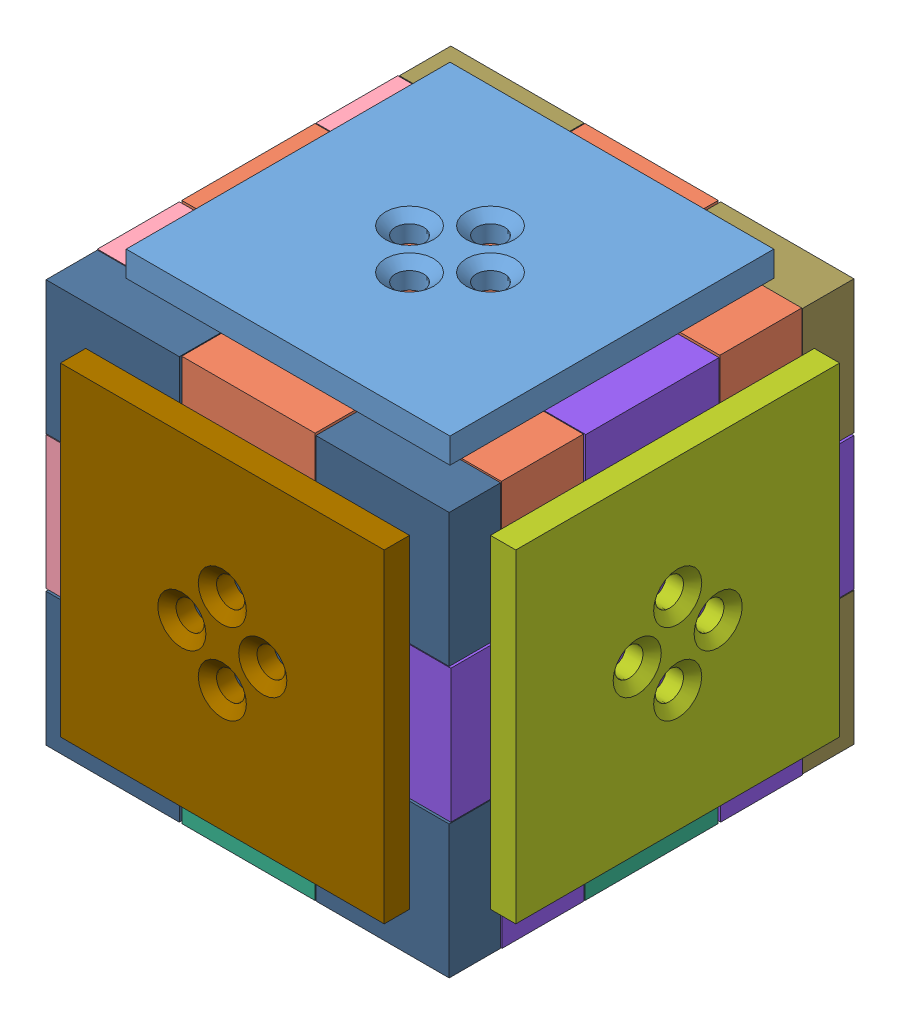
SolidWorks assembly cube_13, configuration cube13. Lengths in mm.
Overall size (28.57 28.57 28.57).
12 component instances, 12 part files, 6 mates.
Components (placement in the parent):
- panel_R^cube_13-13: panel_R^cube_13 [cube01] x (-1 0 0) z (0 0 1) size (20.32 1.59 20.32) (virtual)
- acrylic_R^cube_13-1: acrylic_R^cube_13 [A] at origin size (25.3 3.23 25.3) (virtual)
- panel_O^cube_13-8: panel_O^cube_13 [cube01] x (0 -1 0) z (0 0 1) size (20.32 1.59 20.32) (virtual)
- acrylic_O^cube_13-23: acrylic_O^cube_13 [A] x (0 1 0) z (0 0 1) size (25.3 3.23 25.3) (virtual)
- panel_Y^cube_13-9: panel_Y^cube_13 [cube01] at origin size (20.32 1.59 20.32) (virtual)
- acrylic_Y^cube_13-24: acrylic_Y^cube_13 [A] x (-1 0 0) z (0 0 1) size (25.3 3.23 25.3) (virtual)
- panel_G^cube_13-10: panel_G^cube_13 [cube01] x (0 1 0) z (0 0 1) size (20.32 1.59 20.32) (virtual)
- acrylic_G^cube_13-25: acrylic_G^cube_13 [A] x (0 -1 0) z (0 0 1) size (25.3 3.23 25.3) (virtual)
- panel_C^cube_13-11: panel_C^cube_13 [cube01] x (-1 0 0) z (0 -1 0) size (20.32 1.59 20.32) (virtual)
- acrylic_C^cube_13-26: acrylic_C^cube_13 [B] x (1 0 0) z (0 -1 0) size (25.3 3.23 25.3) (virtual)
- panel_B^cube_13-13: panel_B^cube_13 [cube01] x (-1 0 0) z (0 1 0) size (20.32 1.59 20.32) (virtual)
- acrylic_B^cube_13-27: acrylic_B^cube_13 [B] x (1 0 0) z (0 1 0) size (25.3 3.23 25.3) (virtual)
Mates (geometry in assembly coordinates):
- Coincident1: coincident aligned: plane of panel_R^cube_13-13 through (0 0 0) normal (0 0 1); plane of assembly through (0 0 0) normal (0 0 1)
- Coincident2: coincident anti-aligned: plane of panel_R^cube_13-13; plane of assembly through (0 0 0) normal (1 0 0)
- Coincident3: coincident anti-aligned: plane of panel_R^cube_13-13; plane of assembly through (0 0 0) normal (0 1 0)
- Coincident4: coincident aligned: plane of acrylic_R^cube_13-1 through (0 0 0) normal (0 0 1); plane of assembly through (0 0 0) normal (0 0 1)
- Coincident5: coincident aligned: plane of acrylic_R^cube_13-1 through (0 0 0) normal (1 0 0); plane of assembly through (0 0 0) normal (1 0 0)
- Coincident6: coincident aligned: plane of ? through (0 0 0) normal (0 1 0); plane of assembly through (0 0 0) normal (0 1 0)
